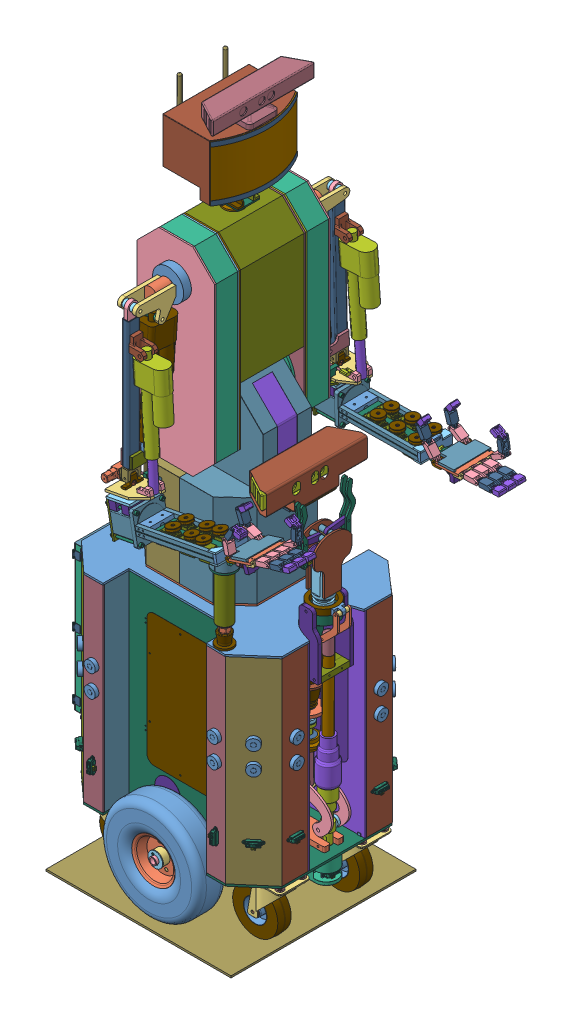
SolidWorks assembly sorbot, configuration По умолчанию. Lengths in mm. (continued)
Mates (geometry in assembly coordinates): (continued)
- Совпадение1280: coincident aligned: plane of SY42STH47-1 through (-54.9903 1468.2936 -152.0542) normal (-1 0 0); plane of head.tilit.p5-1 through (-54.9903 1505.5936 -152.0542) normal (-1 0 0)
- Совпадение1281: coincident anti-aligned: plane of SY42STH47-1 through (-54.9903 1463.2936 -152.0542) normal (0 0 1); plane of head.tilit.p5-1 through (30.0097 1463.2936 -152.0542) normal (0 0 -1)
- Совпадение1283: coincident aligned: plane of head.p1-1 through (-54.9903 1458.2936 -105.9254) normal (-1 0 0); plane of head.tilit.p5-1 through (-54.9903 1505.5936 -152.0542) normal (-1 0 0)
- Заблокировать606: lock: unknown of head.tilt.p1-1; unknown of head.p1-1
- Параллельность222: parallel aligned: plane of body.frame.p2-1 through (92.5097 1112.7235 -222.3642) normal (1 0 0); plane of head.p1-1 through (30.0097 1458.2936 -105.9254) normal (1 0 0)
- Расстояние32: distance = 0.4 mm aligned: plane of head.tilt.p8-1 through (-4.1768 1486.067 -134.1542) normal (0 0 1); plane of head.tilt.p2-1 through (-33.8403 1484.4436 -134.5542) normal (0 0 1)
- Концентричный711: concentric anti-aligned: cylinder of head.tilt.p8-1 through (-4.1768 1486.067 -139.0542) axis (0 0 1) radius 3; cylinder of head.tilt.p9-1 through (-4.1768 1486.067 -112.7074) axis (0 0 -1) radius 3
- Совпадение1286: coincident anti-aligned: plane of head.p1-1 through (30.0097 1458.2936 -164.0542) normal (0 1 0); plane of head.tilit.p5.m-1 through (-54.9903 1458.2936 -121.9254) normal (0 -1 0)
- Совпадение1287: coincident aligned: plane of head.p1-1 through (-54.9903 1458.2936 -105.9254) normal (-1 0 0); plane of head.tilit.p5.m-1 through (-54.9903 1505.5936 -117.9254) normal (-1 0 0)
- Концентричный713: concentric anti-aligned: cylinder of head.tilt.p8-1 through (-4.1768 1486.067 -141.0542) axis (0 0 1) radius 4.85; cylinder of head.tilt.p10-1 through (-4.1768 1486.067 -138.0542) axis (0 0 -1) radius 4.85
- Совпадение1288: coincident anti-aligned: plane of head.tilt.p8-1 through (-4.1768 1486.067 -138.0542) normal (0 0 -1); plane of head.tilt.p10-1 through (-4.1768 1486.067 -138.0542) normal (0 0 1)
- Концентричный714: concentric anti-aligned: cylinder of head.tilt.p8-1 through (-4.1768 1486.067 -132.1542) axis (0 0 -1) radius 4.85; cylinder of head.tilt.p10-2 through (-4.1768 1486.067 -135.1542) axis (0 0 1) radius 4.85
- Совпадение1289: coincident anti-aligned: plane of head.tilt.p8-1 through (-4.1768 1486.067 -135.1542) normal (0 0 1); plane of head.tilt.p10-2 through (-4.1768 1486.067 -135.1542) normal (0 0 -1)
- Концентричный715: concentric anti-aligned: cylinder of head.tilt.p10-2 through (-4.1768 1486.067 -135.1542) axis (0 0 1) radius 4.85; cylinder of head.tilit.p11-1 through (-4.1768 1486.067 -128.1542) axis (0 0 -1) radius 1
- Совпадение1290: coincident anti-aligned: plane of head.tilt.p10-2 through (-4.1768 1486.067 -131.6542) normal (0 0 1); plane of head.tilit.p11-1 through (-6.8677 1566.0217 -131.6542) normal (0 0 -1)
- Концентричный716: concentric aligned: cylinder of head.tilt.p10-1 through (-4.1768 1486.067 -138.0542) axis (0 0 -1) radius 4.85; cylinder of head.tilit.p11-2 through (-4.1768 1486.067 -141.5542) axis (0 0 -1) radius 1
- Совпадение1291: coincident anti-aligned: plane of head.tilt.p10-1 through (-4.1768 1486.067 -141.5542) normal (0 0 -1); plane of head.tilit.p11-2 through (-6.8677 1566.0217 -141.5542) normal (0 0 1)
- Совпадение1292: coincident aligned: plane of head.tilit.p11-1 through (8.1238 1566.5263 -128.1542) normal (0.99746 0.071224 0); plane of head.tilit.p11-2 through (8.1238 1566.5263 -141.5542) normal (0.99746 0.071224 0)
- Заблокировать608: lock: unknown of head.tilt.p8-1; unknown of head.tilt.p10-2
- Заблокировать609: lock: unknown of head.tilt.p8-1; unknown of head.tilt.p10-1
- Заблокировать610: lock: unknown of head.tilt.p10-1; unknown of head.tilit.p11-2
- Заблокировать611: lock: unknown of head.tilt.p10-2; unknown of head.tilit.p11-1
- Концентричный718: concentric anti-aligned: cylinder of head.tilit.p5-1 through (-4.1768 1486.067 -164.0542) axis (0 0 1) radius 3; cylinder of head.tilt.p9-1 through (-4.1768 1486.067 -112.7074) axis (0 0 -1) radius 3
- Концентричный720: concentric aligned: cylinder of head.tilt.p9-1 through (-4.1768 1486.067 -112.7074) axis (0 0 -1) radius 3; cylinder of head.tilt.p12-2 through (-4.1768 1486.067 -145.0542) axis (0 0 -1) radius 3
- Совпадение1294: coincident anti-aligned: plane of head.tilit.p5-1 through (30.0097 1458.2936 -148.0542) normal (0 0 1); plane of head.tilt.p12-2 through (-4.1768 1486.067 -148.0542) normal (0 0 -1)
- Концентричный721: concentric anti-aligned: cylinder of head.tilit.p11-1 through (5.0356 1476.8947 -128.1542) axis (0 0 -1) radius 2; cylinder of m4.nut-5 through (5.0356 1476.8947 -128.1542) axis (0 0 1) radius 2
- Концентричный723: concentric anti-aligned: cylinder of head.tilit.p11-1 through (-4.1485 1473.067 -128.1542) axis (0 0 -1) radius 2; cylinder of m4.nut-6 through (-4.1485 1473.067 -128.1542) axis (0 0 1) radius 2
- Концентричный724: concentric anti-aligned: cylinder of head.tilit.p11-1 through (-13.3492 1476.8546 -128.1542) axis (0 0 -1) radius 2; cylinder of m4.nut-7 through (-13.3492 1476.8546 -128.1542) axis (0 0 1) radius 2
- Концентричный725: concentric anti-aligned: cylinder of head.tilit.p11-1 through (4.9956 1495.2794 -128.1542) axis (0 0 -1) radius 2; cylinder of m4.nut-3 through (4.9956 1495.2794 -128.1542) axis (0 0 1) radius 2
- Концентричный726: concentric anti-aligned: cylinder of head.tilit.p11-1 through (-4.2051 1499.067 -128.1542) axis (0 0 -1) radius 2; cylinder of m4.nut-4 through (-4.2051 1499.067 -128.1542) axis (0 0 1) radius 2
- Концентричный727: concentric anti-aligned: cylinder of head.tilit.p11-1 through (-13.3892 1495.2394 -128.1542) axis (0 0 -1) radius 2; cylinder of m4.nut-8 through (-13.3892 1495.2394 -128.1542) axis (0 0 1) radius 2
- Совпадение1295: coincident anti-aligned: plane of head.tilit.p11-1 through (-6.8677 1566.0217 -128.1542) normal (0 0 1); plane of m4.nut-8 through (-13.3892 1499.2 -128.1542) normal (0 0 -1)
- Совпадение1296: coincident anti-aligned: plane of head.tilit.p11-1 through (-6.8677 1566.0217 -128.1542) normal (0 0 1); plane of m4.nut-4 through (-4.2051 1503.0276 -128.1542) normal (0 0 -1)
- Совпадение1297: coincident anti-aligned: plane of head.tilit.p11-1 through (-6.8677 1566.0217 -128.1542) normal (0 0 1); plane of m4.nut-3 through (4.9956 1499.24 -128.1542) normal (0 0 -1)
- Совпадение1298: coincident anti-aligned: plane of head.tilit.p11-1 through (-6.8677 1566.0217 -128.1542) normal (0 0 1); plane of m4.nut-7 through (-13.3492 1480.8153 -128.1542) normal (0 0 -1)
- Совпадение1299: coincident anti-aligned: plane of head.tilit.p11-1 through (-6.8677 1566.0217 -128.1542) normal (0 0 1); plane of m4.nut-6 through (-4.1485 1477.0277 -128.1542) normal (0 0 -1)
- Совпадение1300: coincident anti-aligned: plane of head.tilit.p11-1 through (-6.8677 1566.0217 -128.1542) normal (0 0 1); plane of m4.nut-5 through (5.0356 1480.8553 -128.1542) normal (0 0 -1)
- Концентричный728: concentric aligned: cylinder of head.tilt.p9-1 through (-4.1768 1486.067 -112.7074) axis (0 0 -1) radius 3; cylinder of m6.washer-7 through (-4.1768 1486.067 -116.2254) axis (0 0 -1) radius 3.25
- Совпадение1301: coincident anti-aligned: plane of head.tilit.p5.m-1 through (-54.9903 1463.2936 -117.9254) normal (0 0 1); plane of m6.washer-7 through (-4.1768 1486.067 -117.9254) normal (0 0 -1)
- Концентричный729: concentric anti-aligned: cylinder of head.tilt.p9-1 through (-4.1768 1486.067 -112.7074) axis (0 0 -1) radius 3; cylinder of m6.washer-8 through (-4.1768 1486.067 -153.7542) axis (0 0 1) radius 3.25
- Совпадение1302: coincident anti-aligned: plane of head.tilit.p5-1 through (30.0097 1463.2936 -152.0542) normal (0 0 -1); plane of m6.washer-8 through (-4.1768 1486.067 -152.0542) normal (0 0 1)
- Заблокировать612: lock: unknown of head.tilit.p5-1; unknown of head.tilt.p9-1
- Концентричный730: concentric aligned: cylinder of head.tilt.p9-1 through (-4.1768 1486.067 -112.7074) axis (0 0 -1) radius 3; cylinder of head.tilt.p12.m-1 through (-4.1768 1486.067 -121.6542) axis (0 0 -1) radius 3
- Совпадение1303: coincident anti-aligned: plane of head.tilit.p11-1 through (-6.8677 1566.0217 -128.1542) normal (0 0 1); plane of head.tilt.p12.m-1 through (-4.1768 1486.067 -128.1542) normal (0 0 -1)
- Совпадение1304: coincident aligned: plane of head.p1-1 through (-54.9903 1458.2936 -105.9254) normal (0 0 1); plane of head.tilit.p5.m-1 through (-54.9903 1463.2936 -105.9254) normal (0 0 1)
- Совпадение1305: coincident aligned: plane of head.p1-1 through (-54.9903 1458.2936 -164.0542) normal (0 0 -1); plane of head.tilit.p5-1 through (30.0097 1463.2936 -164.0542) normal (0 0 -1)
- Концентричный731: concentric anti-aligned: cylinder of head.tilit.p11-1 through (-6.8677 1566.0217 -128.1542) axis (0 0 -1) radius 15; cylinder of head.tilt.p13-1 through (-6.8677 1566.0217 -183.9806) axis (0 0 1) radius 15
- Совпадение1306: coincident anti-aligned: plane of head.tilit.p11-1 through (-6.8677 1566.0217 -131.6542) normal (0 0 -1); plane of head.tilt.p13-1 through (-6.8677 1566.0217 -131.6542) normal (0 0 1)
- Концентричный732: concentric aligned: cylinder of head.p3-1 through (-6.8677 1566.0217 -114.1542) axis (0 0 -1) radius 15.102; cylinder of head.tilit.p11-1 through (-6.8677 1566.0217 -128.1542) axis (0 0 -1) radius 15
- Совпадение1307: coincident anti-aligned: plane of head.tilit.p11-1 through (-6.8677 1566.0217 -128.1542) normal (0 0 1); plane of head.p3-1 through (-21.8677 1551.1571 -128.1542) normal (0 0 -1)
- Концентричный733: concentric anti-aligned: cylinder of head.tilit.p11-2 through (-6.8677 1566.0217 -141.5542) axis (0 0 -1) radius 15; cylinder of head.p3-2 through (-6.8677 1566.0217 -159.0542) axis (0 0 1) radius 15.102
- Совпадение1308: coincident anti-aligned: plane of head.tilit.p11-2 through (-6.8677 1566.0217 -145.0542) normal (0 0 -1); plane of head.p3-2 through (8.1323 1551.1571 -145.0542) normal (0 0 1)
- Совпадение1309: coincident anti-aligned: plane of head.tilit.p11-2 through (-6.8677 1566.0217 -145.0542) normal (0 0 -1); plane of head.p2-1 through (-23.5768 1549.1571 -145.0542) normal (0 0 1)
- Совпадение1311: coincident anti-aligned: plane of head.p3-1 through (-21.8677 1549.1571 -126.1542) normal (0 -1 0); plane of head.p2-1 through (38.3461 1549.1571 -213.999) normal (0 1 0)
- Совпадение1312: coincident: plane of head.tilit.p11-1 through (8.1238 1566.5263 -128.1542) normal (0.99746 0.071224 0); line of head.p2-1 through (9.3641 1549.1571 -128.0542) axis (0 0 -1)
- Заблокировать614: lock: unknown of head.tilit.p11-1; unknown of head.p3-1
- Заблокировать615: lock: unknown of head.tilit.p11-2; unknown of head.p3-2
- Заблокировать616: lock: unknown of head.p2-1; unknown of logitech.sphere.af-1
- Заблокировать617: lock: unknown of head.p2-1; unknown of logitech.sphere.af-2
- Параллельность225: parallel aligned: plane of head.p2-1 through (39.4049 1529.1684 -213.999) normal (0 1 0); plane of head.glass-1 through (-136.7624 1647.1684 -136.5542) normal (0 1 0)
- Расстояние33: distance = 30 mm aligned: plane of head.p2-1 through (39.4049 1527.1684 -213.999) normal (0 -1 0); plane of head.glass-1 through (-136.7624 1497.1684 -136.5542) normal (0 -1 0)
- Концентричный735: concentric aligned: cylinder of head.p2-1 through (23.3461 1547.1571 -198.999) axis (0 1 0) radius 5; circle of logitech.sphere.af-2
- Концентричный736: concentric aligned: cylinder of head.p2-1 through (23.3461 1547.1571 -74.1093) axis (0 1 0) radius 5; circle of logitech.sphere.af-1
- Касательный55: tangent aligned: unknown of logitech.sphere.af-2; cylinder of head.glass-1 through (-136.7624 1647.1684 -136.5542) axis (0 -1 0) radius 211.7321
- Касательный56: tangent aligned: unknown of logitech.sphere.af-1; cylinder of head.glass-1 through (-136.7624 1647.1684 -136.5542) axis (0 -1 0) radius 211.7321
- Расстояние34: distance = 38.4 mm: plane of head.p2-1 through (-26.0264 1529.1684 -59.1093) normal (0 0 1); line of head.glass-1 through (40.4676 1647.1684 -20.7093) axis (0 -1 0)
- Заблокировать618: lock: unknown of head.p2-1; unknown of head.glass-1
- Параллельность226: parallel aligned: plane of head.p1-1 through (30.0097 1458.2936 -105.9254) normal (1 0 0); plane of head.p2-1 through (38.3461 1549.1571 -59.1093) normal (1 0 0)
- Концентричный737: concentric anti-aligned: cylinder of head.glass-1 through (-137.8212 1667.1571 -136.5542) axis (0 -1 0) radius 214.7321; cylinder of head.glass.fixture-1 through (-137.8213 1517.1571 -136.5542) axis (0 1 0) radius 214.7321
- Концентричный738: concentric anti-aligned: cylinder of head.glass-1 through (-137.8212 1667.1571 -136.5542) axis (0 -1 0) radius 214.7321; cylinder of head.glass.fixture-2 through (-137.8212 1655.1571 -136.5542) axis (0 1 0) radius 214.7321
- Совпадение1313: coincident aligned: plane of head.glass-1 through (-137.8212 1667.1571 -136.5542) normal (0 1 0); plane of head.glass.fixture-2 through (-137.8212 1667.1571 -136.5542) normal (0 1 0)
- Совпадение1314: coincident aligned: plane of head.glass-1 through (41.9199 1667.1571 -19.0679) normal (-0.547129 0 0.837048); plane of head.glass.fixture-2 through (41.9199 1655.1571 -19.0679) normal (-0.547129 0 0.837048)
- Совпадение1315: coincident aligned: plane of head.glass-1 through (-137.8213 1517.1571 -136.5542) normal (0 -1 0); plane of head.glass.fixture-1 through (-137.8213 1517.1571 -136.5542) normal (0 -1 0)
- Совпадение1316: coincident aligned: plane of head.glass-1 through (41.9199 1667.1571 -19.0679) normal (-0.547129 0 0.837048); plane of head.glass.fixture-1 through (41.9199 1517.1571 -19.0679) normal (-0.547129 0 0.837048)
- Концентричный739: concentric anti-aligned: cylinder of head.glass-1 through (-137.8212 1667.1571 -136.5542) axis (0 -1 0) radius 211.7321; cylinder of head.p4-1 through (-137.8213 1517.1571 -136.5542) axis (0 1 0) radius 211.73
- Совпадение1317: coincident aligned: plane of head.glass-1 through (-137.8213 1517.1571 -136.5542) normal (0 -1 0); plane of head.p4-1 through (-137.8213 1517.1571 -136.5542) normal (0 -1 0)
- Заблокировать619: lock: unknown of head.p2-1; unknown of head.p4-1
- Совпадение1319: coincident anti-aligned: plane of head.p4-1 through (-84.6104 1578.1571 -252.4244) normal (-1 0 0); plane of ant-3 through (-84.6104 1643.7707 -74.539) normal (1 0 0)
- Совпадение1321: coincident anti-aligned: plane of head.p4-1 through (-84.6104 1578.1571 -252.4244) normal (-1 0 0); plane of ant-2 through (-84.6104 1643.7707 -198.1028) normal (1 0 0)
- Параллельность229: parallel aligned: plane of head.p4-1 through (39.3896 1666.1571 -253.5244) normal (0 0 -1); plane of ant-2 through (-96.1462 1641.4075 -199.6028) normal (0 0 -1)
- Параллельность230: parallel aligned: plane of head.p4-1 through (39.3896 1666.1571 -253.5244) normal (0 0 -1); plane of ant-3 through (-96.1462 1641.4075 -76.039) normal (0 0 -1)
- Заблокировать622: lock: unknown of ant-3; unknown of head.p4-1
- Заблокировать623: lock: unknown of head.p4-1; unknown of ant-2
- Параллельность231: parallel: plane of kinect-black-1 through (-305.9508 1681.1571 -96.5839) normal (0 0 1); plane of head.p4-1 through (-86.6104 1667.1571 -19.5839) normal (0 0 1)
- Совпадение1322: coincident: plane of head.p4-1 through (-137.3095 1668.1571 -136.5542) normal (0 1 0); plane of kinect-black-1 through (-305.9508 1668.1571 -166.5839) normal (0 -1 0)
- Расстояние35: distance = 77 mm aligned: plane of kinect-black-1 through (-305.9508 1681.1571 -96.5839) normal (0 0 1); plane of head.p4-1 through (-86.6104 1667.1571 -19.5839) normal (0 0 1)
- Заблокировать624: lock: unknown of head.p4-1; unknown of kinect-black-1
- Параллельность232: parallel aligned: plane of wall11-1 through (-275.9003 882.565 11.9312) normal (-1 0 0); plane of turret.table-1 through (-172.5648 612.7934 -218.9555) normal (-1 0 0)
- Совпадение1329: coincident aligned: plane of body_pivot-2 through (-90.0648 982.0246 -71.9555) normal (0 0 1); plane of body.cover-1 through (-20.0648 1083.2934 -71.9555) normal (0 0 1)
- Расстояние43: distance = 470 mm: plane of body.cover-1 through (49.9352 1082.7934 -201.9555) normal (0 -1 0); plane of turret.table-1 through (-20.0648 612.7934 -360.2969) normal (0 1 0)
- Coincident1: coincident anti-aligned: plane of wall6-1 through (267.1742 655.3334 -58.2424) normal (1 0 0); plane of Sharp IR GP2D120-1/Sharp IR Body-1 through (267.1742 145.9368 -37.6736) normal (-1 0 0)
- Distance2: distance = 94 mm: line of Sharp IR GP2D120-1/Sharp IR Body-1 through (267.1742 145.9368 -28.4236) axis (0 0 -1); line of wall6-1 through (267.1742 51.9368 11.8264) axis (0 0 -1)
- Distance3: distance = 20 mm: line of wall6-1 through (267.1742 585.1505 11.8264) axis (0 -1 0); line of Sharp IR GP2D120-1/Sharp IR Body-1 through (267.1742 158.9368 -8.1736) axis (0 -1 0)
- Distance6: distance = 20 mm: line of wall7-3 through (267.1973 585.1505 -285.6811) axis (0 -1 0); plane of ? through (274.3242 158.9368 -265.6811) normal (0 0 -1)
- Coincident3: coincident anti-aligned: plane of wall7-3 through (267.1973 693.5591 -285.6811) normal (0.650583 0 -0.759435); plane of Sharp IR GP2D120-3/Sharp IR Body-1 through (214.8514 145.9368 -330.5241) normal (-0.650583 0 0.759435)
- Distance7: distance = 94 mm: line of wall7-3 through (267.1973 51.9368 -285.6811) axis (-0.759435 0 -0.650583); plane of Sharp IR GP2D120-3/Sharp IR Body-1 through (241.9064 145.9368 -316.7619) normal (0 -1 0)
- Lock1: lock: unknown of bottom-2; unknown of wall7-1
- Coincident5: coincident anti-aligned: plane of wall7-1 through (184.8921 693.5591 82.4377) normal (0.650583 0 0.759435); plane of Sharp IR GP2D120-4/Sharp IR Body-1 through (236.9707 145.9368 37.8238) normal (-0.650583 0 -0.759435)
- Distance9: distance = 94 mm: line of wall7-1 through (184.8921 51.9368 82.4377) axis (0.759435 0 -0.650583); plane of Sharp IR GP2D120-4/Sharp IR Body-1 through (219.219 145.9368 62.4459) normal (0 -1 0)
- Coincident8: coincident: plane of wall8-2 through (132.798 -0.3194 -356.1821) normal (0 0 -1); plane of ? through (152.9241 165.4368 -356.1821) normal (0 0 1)
- Distance13: distance = 84 mm: line of wall8-2 through (132.798 51.9368 -356.1821) axis (1 0 0); plane of ? through (165.9241 135.9368 -363.3321) normal (0 -1 0)
- Distance14: distance = 19 mm: line of wall7-3 through (184.9241 585.1505 -356.1619) axis (0 -1 0); plane of ? through (165.9241 135.9368 -363.3321) normal (1 0 0)
- Lock2: lock: unknown of wall8-2; unknown of ?
- Lock3: lock: unknown of wall7-3; unknown of Sharp IR GP2D120-3/Sharp IR Body-1
- Lock4: lock: unknown of wall6-3; unknown of ?
- Lock5: lock: unknown of wall6-1; unknown of Sharp IR GP2D120-1/Sharp IR Body-1
- Lock6: lock: unknown of wall7-1; unknown of Sharp IR GP2D120-4/Sharp IR Body-1
- Lock7: lock: unknown of wall8-1; unknown of Sharp IR GP2D120-5/Sharp IR Body-1
- Lock8: lock: unknown of wall8-5; unknown of ?
- Coincident10: coincident: plane of wall8-4 through (-146.6756 -0.3194 82.4522) normal (0 0 1); plane of Sharp IR GP2D120-8/Sharp IR Body-1 through (-167.0366 165.4368 82.4522) normal (0 0 -1)
- Distance17: distance = 84 mm: line of wall8-4 through (-146.6756 51.9368 82.4522) axis (-1 0 0); plane of Sharp IR GP2D120-8/Sharp IR Body-1 through (-180.0366 135.9368 89.6022) normal (0 -1 0)
- Distance18: distance = 19 mm: line of wall7-v1-1 through (-199.0366 51.9368 82.0998) axis (0 1 0); plane of Sharp IR GP2D120-8/Sharp IR Body-1 through (-180.0366 135.9368 89.6022) normal (-1 0 0)
- Lock9: lock: unknown of wall8-4; unknown of Sharp IR GP2D120-8/Sharp IR Body-1
- Coincident11: coincident: plane of wall7-v1-2 through (-275.6816 -52.2153 -285.955) normal (-0.67421 0 -0.73854); plane of Sharp IR GP2D120-9/Sharp IR Body-1 through (-246.8786 145.9368 -312.2492) normal (0.67421 0 0.73854)
- Distance19: distance = 94 mm: plane of Sharp IR GP2D120-9/Sharp IR Body-1 through (-229.9122 145.9368 -337.419) normal (0 -1 0); line of wall7-v1-2 through (-275.6816 51.9368 -285.955) axis (0.73854 0 -0.67421)
- Distance20: distance = 39 mm: line of wall7-v1-2 through (-275.6816 51.9368 -285.955) axis (0 1 0); plane of Sharp IR GP2D120-9/Sharp IR Body-1 through (-251.6992 158.9368 -317.5298) normal (-0.73854 0 0.67421)
- Lock10: lock: unknown of wall7-v1-2; unknown of Sharp IR GP2D120-9/Sharp IR Body-1
- Coincident12: coincident anti-aligned: plane of wall7-v1-1 through (-199.0366 -52.2153 82.0998) normal (-0.67421 0 0.73854); plane of Sharp IR GP2D120-10/Sharp IR Body-1 through (-225.3104 145.9368 58.1146) normal (0.67421 0 -0.73854)
- Distance21: distance = 94 mm: plane of Sharp IR GP2D120-10/Sharp IR Body-1 through (-251.9179 145.9368 43.5059) normal (0 -1 0); line of bottom-2 through (-275.9596 51.9368 11.9714) axis (0.73854 0 0.67421)
- Distance22: distance = 39 mm: line of wall7-v1-1 through (-275.9003 51.9368 11.9312) axis (0 1 0); plane of Sharp IR GP2D120-10/Sharp IR Body-1 through (-251.9179 158.9368 43.5059) normal (-0.73854 0 -0.67421)
- Lock11: lock: unknown of wall7-v1-1; unknown of Sharp IR GP2D120-10/Sharp IR Body-1
- Coincident13: coincident anti-aligned: plane of wall10-v1-1 through (132.8227 864.7556 -286.1821) normal (0 0 -1); plane of wall10.opening.cap-1 through (52.686 120.491 -286.1821) normal (0 0 1)
- Concentric1: concentric aligned: circle of wall10-v1-1; circle of wall10.opening.cap-1
- Coincident14: coincident anti-aligned: plane of wall10-1 through (-146.6756 864.7556 12.4522) normal (0 0 1); plane of wall10.opening.cap-2 through (-41.2841 118.8489 12.4522) normal (0 0 -1)
- Concentric2: concentric aligned: circle of wall10-1; circle of wall10.opening.cap-2
- Coincident15: coincident anti-aligned: plane of wall10-1 through (-146.6756 864.7556 12.4522) normal (0 0 1); plane of wall10-cap-1 through (-77.6414 499.1505 12.4522) normal (0 0 -1)
- Coincident16: coincident anti-aligned: plane of wall10-v1-1 through (132.8227 864.7556 -286.1821) normal (0 0 -1); plane of wall10-cap-2 through (-77.5708 499.1505 -286.1821) normal (0 0 1)
- Coincident17: coincident anti-aligned: plane of wall6-1 through (267.1742 655.3334 -58.2424) normal (1 0 0); plane of us_sensor-1 through (267.1742 386.9368 -23.208) normal (-1 0 0)
- Coincident18: coincident anti-aligned: plane of bottom-2 through (-49.3372 51.9368 -286.1821) normal (0 1 0); plane of wall6-3 through (263.1741 51.9368 -286.3112) normal (0 -1 0)
- Coincident19: coincident aligned: line of wall2-2 through (267.1741 585.1505 -216.2424) axis (0 -1 0); line of wall6-3 through (267.1741 585.1505 -216.2424) axis (0 -1 0)
- Coincident20: coincident aligned: plane of bottom-2 through (267.1742 51.9368 -285.7013) normal (1 0 0); plane of wall6-3 through (267.1741 655.3334 -286.3112) normal (1 0 0)
- Coincident21: coincident anti-aligned: plane of wall6-1 through (267.1742 655.3334 -58.2424) normal (1 0 0); plane of us_sensor-2 through (267.1742 326.9368 -23.208) normal (-1 0 0)
- Concentric3: concentric anti-aligned: cylinder of wall6-1 through (263.1742 386.9368 -23.208) axis (1 0 0) radius 6; cylinder of us_sensor-1 through (277.1742 386.9368 -23.208) axis (-1 0 0) radius 15
- Concentric4: concentric anti-aligned: cylinder of wall6-1 through (263.1742 326.9368 -23.208) axis (1 0 0) radius 6; cylinder of us_sensor-2 through (277.1742 326.9368 -23.208) axis (-1 0 0) radius 15
- Coincident22: coincident anti-aligned: plane of wall6-3 through (267.1742 655.3334 -286.3112) normal (1 0 0); plane of us_sensor-3 through (267.1742 326.9368 -251.2768) normal (-1 0 0)
- Coincident23: coincident anti-aligned: plane of wall6-3 through (267.1742 655.3334 -286.3112) normal (1 0 0); plane of us_sensor-4 through (267.1742 386.9368 -251.2768) normal (-1 0 0)
- Concentric5: concentric anti-aligned: cylinder of wall6-3 through (263.1742 386.9368 -251.2768) axis (1 0 0) radius 6; cylinder of us_sensor-4 through (277.1742 386.9368 -251.2768) axis (-1 0 0) radius 15
- Concentric6: concentric anti-aligned: cylinder of wall6-3 through (263.1742 326.9368 -251.2768) axis (1 0 0) radius 6; cylinder of us_sensor-3 through (277.1742 326.9368 -251.2768) axis (-1 0 0) radius 15
- Coincident24: coincident anti-aligned: plane of bottom-2 through (-49.3372 51.9368 -286.1821) normal (0 1 0); plane of wall8-5 through (-199.1911 51.9368 -356.1821) normal (0 -1 0)
- Coincident26: coincident aligned: plane of bottom-2 through (-146.7539 51.9368 -356.1821) normal (0 0 -1); plane of wall8-5 through (-199.1911 51.9368 -356.1821) normal (0 0 -1)
- Coincident27: coincident aligned: plane of bottom-2 through (-146.7539 51.9368 -286.1821) normal (1 0 0); plane of wall9-3 through (-146.7539 655.1671 -356.1821) normal (1 0 0)
- Lock12: lock: unknown of bottom-2; unknown of wall9-3
- Coincident31: coincident anti-aligned: plane of bottom-2 through (-49.3372 51.9368 -286.1821) normal (0 1 0); plane of wall8-1 through (184.8921 51.9368 82.4377) normal (0 -1 0)
- Coincident32: coincident anti-aligned: line of wall7-1 through (184.8921 585.1505 82.4377) axis (0 -1 0); line of wall8-1 through (184.8921 51.9368 82.4377) axis (0 1 0)
- Coincident34: coincident anti-aligned: plane of wall7-3 through (267.1973 693.5591 -285.6811) normal (0.650583 0 -0.759435); plane of us_sensor-5 through (226.0607 386.9368 -320.9215) normal (-0.650583 0 0.759435)
- Coincident35: coincident anti-aligned: plane of wall7-3 through (267.1973 693.5591 -285.6811) normal (0.650583 0 -0.759435); plane of us_sensor-6 through (226.0607 326.9368 -320.9215) normal (-0.650583 0 0.759435)
- Concentric7: concentric anti-aligned: cylinder of wall7-3 through (223.4584 386.9368 -317.8837) axis (0.650583 0 -0.759435) radius 6; cylinder of us_sensor-5 through (232.5665 386.9368 -328.5158) axis (-0.650583 0 0.759435) radius 15
- Concentric8: concentric anti-aligned: cylinder of wall7-3 through (223.4584 326.9368 -317.8837) axis (0.650583 0 -0.759435) radius 6; cylinder of us_sensor-6 through (232.5665 326.9368 -328.5158) axis (-0.650583 0 0.759435) radius 15
- Coincident36: coincident anti-aligned: plane of wall8-2 through (132.798 51.9368 -356.1821) normal (0 0 -1); plane of us_sensor-8 through (158.8495 386.9368 -356.1821) normal (0 0 1)
- Coincident37: coincident: plane of wall8-2 through (132.798 51.9368 -356.1821) normal (0 0 -1); plane of us_sensor-7 through (158.8495 326.9368 -356.1821) normal (0 0 1)
- Concentric9: concentric anti-aligned: cylinder of wall8-2 through (158.8495 386.9368 -352.1821) axis (0 0 -1) radius 6; cylinder of us_sensor-8 through (158.8495 386.9368 -366.1821) axis (0 0 1) radius 15
- Concentric10: concentric anti-aligned: cylinder of wall8-2 through (158.8495 326.9368 -352.1821) axis (0 0 -1) radius 6; cylinder of us_sensor-7 through (158.8495 326.9368 -366.1821) axis (0 0 1) radius 15
- Coincident38: coincident: plane of wall8-5 through (-199.1911 51.9368 -356.1821) normal (0 0 -1); plane of us_sensor-10 through (-173.1397 386.9368 -356.1821) normal (0 0 1)
- Coincident39: coincident: plane of wall8-5 through (-199.1911 51.9368 -356.1821) normal (0 0 -1); plane of us_sensor-9 through (-173.1397 326.9368 -356.1821) normal (0 0 1)
- Concentric11: concentric anti-aligned: cylinder of wall8-5 through (-173.1397 386.9368 -352.1821) axis (0 0 -1) radius 6; cylinder of us_sensor-10 through (-173.1397 386.9368 -366.1821) axis (0 0 1) radius 15
- Concentric12: concentric anti-aligned: cylinder of wall8-5 through (-173.1397 326.9368 -352.1821) axis (0 0 -1) radius 6; cylinder of us_sensor-9 through (-173.1397 326.9368 -366.1821) axis (0 0 1) radius 15
- Coincident40: coincident: plane of wall7-v1-2 through (-275.6816 -52.2153 -285.955) normal (-0.67421 0 -0.73854); plane of us_sensor-12 through (-237.2497 386.9368 -321.0393) normal (0.67421 0 0.73854)
- Coincident41: coincident: plane of wall7-v1-2 through (-275.6816 -52.2153 -285.955) normal (-0.67421 0 -0.73854); plane of us_sensor-11 through (-237.2497 326.9368 -321.0393) normal (0.67421 0 0.73854)
- Concentric13: concentric anti-aligned: cylinder of wall7-v1-2 through (-234.5529 386.9368 -318.0852) axis (-0.67421 0 -0.73854) radius 6; cylinder of us_sensor-12 through (-243.9918 386.9368 -328.4247) axis (0.67421 0 0.73854) radius 15
- Concentric14: concentric anti-aligned: cylinder of wall7-v1-2 through (-234.5529 326.9368 -318.0852) axis (-0.67421 0 -0.73854) radius 6; cylinder of us_sensor-11 through (-243.9918 326.9368 -328.4247) axis (0.67421 0 0.73854) radius 15
- Coincident42: coincident: plane of wall7-v1-1 through (-199.0366 -52.2153 82.0998) normal (-0.67421 0 0.73854); plane of us_sensor-14 through (-237.4685 386.9368 47.0155) normal (0.67421 0 -0.73854)
- Coincident43: coincident: plane of wall7-v1-1 through (-199.0366 -52.2153 82.0998) normal (-0.67421 0 0.73854); plane of us_sensor-13 through (-237.4685 326.9368 47.0155) normal (0.67421 0 -0.73854)
- Concentric15: concentric anti-aligned: cylinder of wall7-v1-1 through (-234.7716 386.9368 44.0613) axis (-0.67421 0 0.73854) radius 6; cylinder of us_sensor-14 through (-244.2106 386.9368 54.4009) axis (0.67421 0 -0.73854) radius 15
- Concentric16: concentric anti-aligned: cylinder of wall7-v1-1 through (-234.7716 326.9368 44.0613) axis (-0.67421 0 0.73854) radius 6; cylinder of us_sensor-13 through (-244.2106 326.9368 54.4009) axis (0.67421 0 -0.73854) radius 15
- Coincident44: coincident: plane of wall8-4 through (-146.6756 51.9505 82.4522) normal (0 0 1); plane of us_sensor-16 through (-172.7271 386.9505 82.4522) normal (0 0 -1)
- Coincident45: coincident: plane of wall8-4 through (-146.6756 51.9505 82.4522) normal (0 0 1); plane of us_sensor-15 through (-172.7271 326.9505 82.4522) normal (0 0 -1)
- Concentric17: concentric anti-aligned: cylinder of wall8-4 through (-172.7271 386.9505 78.4522) axis (0 0 1) radius 6; cylinder of us_sensor-16 through (-172.7271 386.9505 92.4522) axis (0 0 -1) radius 15
- Concentric18: concentric anti-aligned: cylinder of wall8-4 through (-172.7271 326.9505 78.4522) axis (0 0 1) radius 6; cylinder of us_sensor-15 through (-172.7271 326.9505 92.4522) axis (0 0 -1) radius 15
- Coincident46: coincident: plane of wall8-1 through (184.8921 51.9368 82.4377) normal (-0.006017 0 0.999982); plane of us_sensor-18 through (158.8412 386.9368 82.281) normal (0.006017 0 -0.999982)
- Coincident47: coincident: plane of wall8-1 through (184.8921 51.9368 82.4377) normal (-0.006017 0 0.999982); plane of us_sensor-17 through (158.8412 326.9368 82.281) normal (0.006017 0 -0.999982)
- Concentric19: concentric anti-aligned: cylinder of wall8-1 through (158.8652 386.9368 78.281) axis (-0.006017 0 0.999982) radius 6; cylinder of us_sensor-18 through (158.781 386.9368 92.2808) axis (0.006017 0 -0.999982) radius 15
- Concentric20: concentric anti-aligned: cylinder of wall8-1 through (158.8652 326.9368 78.281) axis (-0.006017 0 0.999982) radius 6; cylinder of us_sensor-17 through (158.781 326.9368 92.2808) axis (0.006017 0 -0.999982) radius 15
- Coincident48: coincident: plane of wall7-1 through (184.8921 693.5591 82.4377) normal (0.650583 0 0.759435); plane of us_sensor-20 through (226.0288 386.9368 47.1973) normal (-0.650583 0 -0.759435)
- Coincident49: coincident: plane of wall7-1 through (184.8921 693.5591 82.4377) normal (0.650583 0 0.759435); plane of us_sensor-19 through (226.0288 326.9368 47.1973) normal (-0.650583 0 -0.759435)
- Concentric21: concentric anti-aligned: cylinder of wall7-1 through (223.4265 386.9368 44.1596) axis (0.650583 0 0.759435) radius 6; cylinder of us_sensor-20 through (232.5346 386.9368 54.7917) axis (-0.650583 0 -0.759435) radius 15
- Concentric22: concentric anti-aligned: cylinder of wall7-1 through (223.4265 326.9368 44.1596) axis (0.650583 0 0.759435) radius 6; cylinder of us_sensor-19 through (232.5346 326.9368 54.7917) axis (-0.650583 0 -0.759435) radius 15
- Lock13: lock: unknown of wall6-3; unknown of us_sensor-4
- Lock14: lock: unknown of wall6-3; unknown of us_sensor-3
- Lock15: lock: unknown of wall7-3; unknown of us_sensor-5
- Lock16: lock: unknown of wall7-3; unknown of us_sensor-6
- Lock17: lock: unknown of wall8-2; unknown of us_sensor-8
- Lock18: lock: unknown of wall8-2; unknown of us_sensor-7
- Lock19: lock: unknown of wall8-5; unknown of us_sensor-10
- Lock20: lock: unknown of wall8-5; unknown of us_sensor-9
- Lock21: lock: unknown of wall7-v1-2; unknown of us_sensor-12
- Lock22: lock: unknown of wall7-v1-2; unknown of us_sensor-11
- Lock23: lock: unknown of wall7-v1-1; unknown of us_sensor-14
- Lock24: lock: unknown of wall7-v1-1; unknown of us_sensor-13
- Lock25: lock: unknown of wall8-4; unknown of us_sensor-16
- Lock26: lock: unknown of wall8-4; unknown of us_sensor-15
- Lock27: lock: unknown of wall8-1; unknown of us_sensor-18
- Lock28: lock: unknown of wall8-1; unknown of us_sensor-17
- Lock29: lock: unknown of wall7-1; unknown of us_sensor-20
- Lock30: lock: unknown of wall7-1; unknown of us_sensor-19
- Lock31: lock: unknown of wall6-1; unknown of us_sensor-1
- Lock32: lock: unknown of wall6-1; unknown of us_sensor-2
- Coincident50: coincident: plane of wall11-1 through (-271.9003 882.565 10.1667) normal (1 0 0); plane of computer.box.hinge-1 through (-271.9003 559.9368 -55.5688) normal (-1 0 0)
- Coincident51: coincident: plane of wall11-1 through (-271.9003 882.565 10.1667) normal (1 0 0); plane of computer.box.hinge-2 through (-271.9003 559.9368 -217.9564) normal (-1 0 0)
- Coincident52: coincident: point of wall11-1; unknown of computer.box.hinge-2
- Coincident53: coincident: unknown of wall11-1; unknown of computer.box.hinge-1
- Lock33: lock: unknown of wall11-1; unknown of computer.box.hinge-1
- Lock34: lock: unknown of wall11-1; unknown of computer.box.hinge-2
- Lock36: lock: unknown of computer.box.hinge-2; unknown of computer.box.console-1/computer.box.fixture.console-1
- Coincident58: coincident anti-aligned: plane of wall11-1 through (-271.9003 556.9368 -38.0688) normal (0 1 0); plane of computer.box.console-2/cap-hinge-p1-1 through (-280.8434 556.9368 -36.0276) normal (0 -1 0)
- Lock37: lock: unknown of computer.box.hinge-1; unknown of computer.box.console-2/computer.box.fixture.console-1
- Concentric23: concentric anti-aligned: cylinder of computer.box.console-2/cap-hinge-p1-1 through (-280.8434 559.9368 -36.0276) axis (0 0 -1) radius 2; cylinder of computer.box.base-1/cap-hinge-2 through (-280.8434 559.9368 -75.2651) axis (0 0 1) radius 2
- Coincident60: coincident anti-aligned: plane of computer.box.console-2/cap-hinge-p1-1 through (-275.9003 539.9368 -65.2651) normal (0 0 -1); plane of computer.box.base-1/cap-hinge-2 through (-260.8434 565.7704 -65.2651) normal (0 0 1)
- Coincident67: coincident anti-aligned: plane of computer.box.base-1/computer.box.cap.hinge.p2-1 through (-311.8434 354.9938 -4.6907) normal (0 -1 0); plane of computer.box.cap-1/computer.box.cap.hinge.p1-2 through (-317.3839 354.9938 1.7687) normal (0 1 0)
- Concentric27: concentric anti-aligned: cylinder of computer.box.base-1/computer.box.cap.hinge.p2-1 through (-315.7839 349.9938 -6.2907) axis (0 1 0) radius 1; cylinder of computer.box.cap-1/computer.box.cap.hinge.p1-2 through (-315.7839 369.9938 -6.2907) axis (0 -1 0) radius 1
- Parallel2: parallel aligned: plane of wall11-1 through (-275.9003 882.565 11.9312) normal (-1 0 0); unknown of computer.box.cap-1/computer.box.cap.base-1
- Lock39: lock: unknown of computer.box.base-1/computer.box.corner.p1-2; unknown of computer.box.cap-1/computer.box.cap.base-1
- Parallel1: parallel anti-aligned: plane of wall11-1 through (-275.9003 882.565 11.9312) normal (-1 0 0); plane of computer.box.base-1/computer.box.bottom-1 through (-281.8434 357.9938 -137.7651) normal (1 0 0)
- Coincident68: coincident anti-aligned: plane of bottom-2 through (-49.3372 51.9368 -286.1821) normal (0 1 0); plane of accumulator.5Ah-2 through (-152.9596 51.9368 -134.0478) normal (0 -1 0)
- Parallel3: parallel aligned: plane of bottom-2 through (-275.9596 51.9368 -285.7013) normal (-1 0 0); plane of accumulator.5Ah-2 through (-235.9596 53.9368 -68.0478) normal (-1 0 0)
- Distance23: distance = 40 mm aligned: plane of bottom-2 through (-275.9596 51.9368 -285.7013) normal (-1 0 0); plane of accumulator.5Ah-2 through (-235.9596 53.9368 -68.0478) normal (-1 0 0)
- Distance24: distance = 148.5 mm aligned: plane of bottom-2 through (-146.7539 51.9368 82.4522) normal (0 0 1); plane of accumulator.5Ah-2 through (-152.9596 139.9368 -66.0478) normal (0 0 1)
- Coincident69: coincident anti-aligned: plane of bottom-2 through (-49.3372 51.9368 -286.1821) normal (0 1 0); plane of accumulator.5Ah-1 through (-152.9596 51.9368 -205.6821) normal (0 -1 0)
- Distance25: distance = 40 mm aligned: plane of accumulator.5Ah-1 through (-235.9596 53.9368 -139.6821) normal (-1 0 0); plane of bottom-2 through (-275.9596 51.9368 -285.7013) normal (-1 0 0)
- Distance26: distance = 148.5 mm aligned: plane of accumulator.5Ah-1 through (-152.9596 139.9368 -207.6821) normal (0 0 -1); plane of bottom-2 through (-146.7539 51.9368 -356.1821) normal (0 0 -1)
- Parallel4: parallel aligned: plane of bottom-2 through (-275.9596 51.9368 -285.7013) normal (-1 0 0); plane of accumulator.loft-1 through (-270.9596 147.9368 -244.8821) normal (-1 0 0)
- Distance27: distance = 91 mm anti-aligned: plane of accumulator.loft-1 through (-267.9596 142.9368 -244.8821) normal (0 -1 0); plane of bottom-2 through (-49.3372 51.9368 -286.1821) normal (0 1 0)
- Distance28: distance = 108.3 mm aligned: plane of bottom-2 through (-146.7539 51.9368 -356.1821) normal (0 0 -1); plane of accumulator.loft-1 through (-108.9596 147.9368 -247.8821) normal (0 0 -1)
- Distance29: distance = 5 mm aligned: plane of bottom-2 through (-275.9596 51.9368 -285.7013) normal (-1 0 0); plane of accumulator.loft-1 through (-270.9596 147.9368 -244.8821) normal (-1 0 0)
- Coincident70: coincident anti-aligned: plane of accumulator.loft-1 through (-267.9596 142.9368 -244.8821) normal (0 -1 0); plane of accumulator.loft.pillar-1 through (-117.9596 142.9368 -39.8821) normal (0 1 0)
- Coincident71: coincident anti-aligned: plane of accumulator.loft-1 through (-267.9596 142.9368 -244.8821) normal (0 -1 0); plane of accumulator.loft.pillar-2 through (-225.9596 142.9368 -39.8821) normal (0 1 0)
- Coincident72: coincident anti-aligned: plane of accumulator.loft-1 through (-267.9596 142.9368 -244.8821) normal (0 -1 0); plane of accumulator.loft.pillar-3 through (-117.9596 142.9368 -235.8821) normal (0 1 0)
- Coincident73: coincident anti-aligned: plane of accumulator.loft-1 through (-267.9596 142.9368 -244.8821) normal (0 -1 0); plane of accumulator.loft.pillar-4 through (-225.9596 142.9368 -235.8821) normal (0 1 0)
- Concentric28: concentric aligned: cylinder of accumulator.loft-1 through (-117.9596 147.9368 -39.8821) axis (0 -1 0) radius 2.5; cylinder of accumulator.loft.pillar-1 through (-117.9596 142.9368 -39.8821) axis (0 -1 0) radius 3
- Concentric29: concentric aligned: cylinder of accumulator.loft-1 through (-225.9596 147.9368 -39.8821) axis (0 -1 0) radius 2.5; cylinder of accumulator.loft.pillar-2 through (-225.9596 142.9368 -39.8821) axis (0 -1 0) radius 3
- Concentric30: concentric aligned: cylinder of accumulator.loft-1 through (-117.9596 147.9368 -235.8821) axis (0 -1 0) radius 2.5; cylinder of accumulator.loft.pillar-3 through (-117.9596 142.9368 -235.8821) axis (0 -1 0) radius 3
- Concentric31: concentric aligned: cylinder of accumulator.loft-1 through (-225.9596 147.9368 -235.8821) axis (0 -1 0) radius 2.5; cylinder of accumulator.loft.pillar-4 through (-225.9596 142.9368 -235.8821) axis (0 -1 0) radius 3
- Coincident74: coincident anti-aligned: plane of accumulator.loft-1 through (-267.9596 147.9368 -244.8821) normal (0 1 0); plane of accumulator.loft.rubber-1 through (-188.4596 147.9368 -137.8821) normal (0 -1 0)
- Parallel5: parallel aligned: plane of accumulator.loft-1 through (-270.9596 147.9368 -244.8821) normal (-1 0 0); plane of accumulator.loft.rubber-1 through (-269.9596 154.9368 -246.8821) normal (-1 0 0)
- Distance31: distance = 1 mm aligned: plane of accumulator.loft.rubber-1 through (-106.9596 154.9368 -28.8821) normal (0 0 1); plane of accumulator.loft-1 through (-108.9596 147.9368 -27.8821) normal (0 0 1)
- Distance32: distance = 1 mm aligned: plane of accumulator.loft-1 through (-270.9596 147.9368 -244.8821) normal (-1 0 0); plane of accumulator.loft.rubber-1 through (-269.9596 154.9368 -246.8821) normal (-1 0 0)
- Coincident75: coincident anti-aligned: plane of accumulator1-1 through (-270.9596 154.9368 -27.8821) normal (0 -1 0); plane of accumulator.loft.rubber-1 through (-188.4596 154.9368 -137.8821) normal (0 1 0)
- Coincident78: coincident aligned: plane of accumulator1-1 through (-270.9596 320.9368 -247.8821) normal (-1 0 0); plane of accumulator.loft-1 through (-270.9596 147.9368 -244.8821) normal (-1 0 0)
- Coincident79: coincident aligned: plane of accumulator1-1 through (-105.9596 320.9368 -27.8821) normal (0 0 1); plane of accumulator.loft-1 through (-108.9596 147.9368 -27.8821) normal (0 0 1)
- Coincident80: coincident anti-aligned: plane of wall11-1 through (-275.9003 882.565 11.9312) normal (-1 0 0); plane of us_sensor-21 through (-275.9003 565.1505 -170.4564) normal (1 0 0)
- Coincident81: coincident anti-aligned: plane of wall11-1 through (-275.9003 882.565 11.9312) normal (-1 0 0); plane of us_sensor-22 through (-275.9003 565.1505 -103.0688) normal (1 0 0)
- Coincident82: coincident anti-aligned: plane of wall11-1 through (-275.9003 882.565 11.9312) normal (-1 0 0); plane of us_sensor-23 through (-275.9003 146.9368 -170.4564) normal (1 0 0)
- Coincident83: coincident anti-aligned: plane of wall11-1 through (-275.9003 882.565 11.9312) normal (-1 0 0); plane of us_sensor-24 through (-275.9003 146.9368 -103.0688) normal (1 0 0)
- Concentric32: concentric anti-aligned: cylinder of wall11-1 through (-271.9003 570.1505 -170.4564) axis (-1 0 0) radius 6; cylinder of us_sensor-21 through (-285.9003 570.1505 -170.4564) axis (1 0 0) radius 15
- Concentric33: concentric anti-aligned: cylinder of wall11-1 through (-271.9003 570.1505 -103.0688) axis (-1 0 0) radius 6; cylinder of us_sensor-22 through (-285.9003 570.1505 -103.0688) axis (1 0 0) radius 15
- Concentric34: concentric anti-aligned: cylinder of wall11-1 through (-271.9003 146.9368 -170.4564) axis (-1 0 0) radius 6; cylinder of us_sensor-23 through (-285.9003 146.9368 -170.4564) axis (1 0 0) radius 15
- Concentric35: concentric anti-aligned: cylinder of wall11-1 through (-271.9003 146.9368 -103.0688) axis (-1 0 0) radius 6; cylinder of us_sensor-24 through (-285.9003 146.9368 -103.0688) axis (1 0 0) radius 15
- Coincident84: coincident anti-aligned: plane of wall11-1 through (-275.9003 882.565 11.9312) normal (-1 0 0); plane of ? through (-275.9003 145.9368 101.8971) normal (1 0 0)
- Coincident85: coincident anti-aligned: plane of wall11-1 through (-275.9003 882.565 11.9312) normal (-1 0 0); plane of ? through (-275.9003 145.9368 145.8787) normal (1 0 0)
- Parallel6: parallel anti-aligned: plane of bottom-2 through (-49.3372 51.9368 -286.1821) normal (0 1 0); plane of ? through (-283.0503 145.9368 72.3971) normal (0 -1 0)
- Parallel7: parallel anti-aligned: plane of bottom-2 through (-49.3372 51.9368 -286.1821) normal (0 1 0); plane of ? through (-283.0503 145.9368 116.3787) normal (0 -1 0)
- Distance33: distance = 94 mm: line of bottom-2 through (-275.9596 51.9368 -285.7013) axis (0 0 1); plane of Sharp IR GP2D120-11/Sharp IR Body-1 through (-283.0503 145.9368 -245.4564) normal (0 -1 0)
- Distance34: distance = 94 mm: plane of Sharp IR GP2D120-12/Sharp IR Body-1 through (-283.0503 145.9368 -57.5688) normal (0 -1 0); line of bottom-2 through (-275.9596 51.9368 -285.7013) axis (0 0 1)
- Distance35: distance = 40 mm: line of wall11-1 through (-275.9003 585.1505 -285.4564) axis (0 -1 0); plane of Sharp IR GP2D120-11/Sharp IR Body-1 through (-283.0503 158.9368 -245.4564) normal (0 0 -1)
- Distance36: distance = 40 mm: line of wall11-1 through (-275.9003 585.1505 11.9312) axis (0 -1 0); plane of Sharp IR GP2D120-12/Sharp IR Body-1 through (-283.0503 158.9368 -28.0688) normal (0 0 1)
- Lock40: lock: unknown of wall11-1; unknown of us_sensor-21
- Lock41: lock: unknown of wall11-1; unknown of us_sensor-22
- Lock42: lock: unknown of wall11-1; unknown of us_sensor-23
- Lock43: lock: unknown of wall11-1; unknown of us_sensor-24
- Lock44: lock: unknown of wall11-1; unknown of Sharp IR GP2D120-11/Sharp IR Body-1
- Lock45: lock: unknown of wall11-1; unknown of Sharp IR GP2D120-12/Sharp IR Body-1
- Coincident86: coincident: unknown of accumulator.charger.sm1236-1; unknown of pillar.10mm-1
- Coincident87: coincident: unknown of accumulator.charger.sm1236-1; unknown of pillar.10mm-2
- Coincident88: coincident: unknown of accumulator.charger.sm1236-1; unknown of pillar.10mm-3
- Coincident89: coincident: unknown of accumulator.charger.sm1236-1; unknown of pillar.10mm-4
- Concentric36: concentric anti-aligned: cylinder of accumulator.charger.sm1236-1 through (-347.0666 292.9966 -370.5276) axis (0 1 0) radius 2; cylinder of pillar.10mm-2 through (-347.0666 292.9966 -370.5276) axis (0 -1 0) radius 1.5
- Concentric37: concentric anti-aligned: cylinder of accumulator.charger.sm1236-1 through (-347.0666 292.9966 -322.0562) axis (0 1 0) radius 2; cylinder of pillar.10mm-3 through (-347.0666 292.9966 -322.0562) axis (0 -1 0) radius 1.5
- Concentric38: concentric anti-aligned: cylinder of accumulator.charger.sm1236-1 through (-538.5098 292.9966 -312.004) axis (0 1 0) radius 2; cylinder of pillar.10mm-1 through (-538.5098 292.9966 -312.004) axis (0 -1 0) radius 1.5
- Concentric39: concentric anti-aligned: cylinder of accumulator.charger.sm1236-1 through (-538.5098 292.9966 -380.5797) axis (0 1 0) radius 2; cylinder of pillar.10mm-4 through (-538.5098 292.9966 -380.5797) axis (0 -1 0) radius 1.5
- Lock46: lock: unknown of accumulator.charger.sm1236-1; unknown of pillar.10mm-4
- Lock47: lock: unknown of accumulator.charger.sm1236-1; unknown of pillar.10mm-1
- Lock48: lock: unknown of accumulator.charger.sm1236-1; unknown of pillar.10mm-3
- Lock49: lock: unknown of accumulator.charger.sm1236-1; unknown of pillar.10mm-2
- Parallel8: parallel anti-aligned: plane of bottom-2 through (-49.3372 51.9368 -286.1821) normal (0 1 0); plane of accumulator.charger.sm1236-1 through (216.0916 329.8029 -262.3065) normal (0 -1 0)
- Coincident91: coincident anti-aligned: plane of wall-fixture-v1-2 through (-152.6756 584.9368 28.4522) normal (-1 0 0); plane of electic.base.plate-1 through (-152.6756 514.1505 -136.5478) normal (1 0 0)
- Parallel9: parallel aligned: plane of wall9-3 through (-142.2412 585.1505 -459.5586) normal (0 1 0); plane of electic.base.plate-1 through (-157.6756 565.1505 34.4522) normal (0 1 0)
- Distance37: distance = 44 mm anti-aligned: plane of wall8-4 through (-146.6756 51.9505 78.4522) normal (0 0 -1); plane of electic.base.plate-1 through (-157.6756 463.1505 34.4522) normal (0 0 1)
- Distance38: distance = 20 mm anti-aligned: plane of cap-1 through (216.6678 585.1505 -83.5666) normal (0 -1 0); plane of electic.base.plate-1 through (-157.6756 565.1505 34.4522) normal (0 1 0)
- Coincident96: coincident anti-aligned: plane of wall-fixture-v2-1-1 through (-269.9003 624.2006 -10.7109) normal (1 0 0); plane of computer.box.screw.fixture-2 through (-269.9003 548.1505 0.207) normal (-1 0 0)
- Coincident97: coincident anti-aligned: plane of wall-fixture-v2-1-2 through (-269.9003 624.1077 -280.8026) normal (1 0 0); plane of computer.box.screw.fixture-1 through (-269.9003 548.1505 -274.4564) normal (-1 0 0)
- Coincident98: coincident anti-aligned: plane of wall-fixture-v2-1-2 through (-269.9003 624.1077 -280.8026) normal (1 0 0); plane of computer.box.screw.fixture-3 through (-269.9003 171.4368 0.207) normal (-1 0 0)
- Coincident99: coincident anti-aligned: plane of wall-fixture-v2-1-1 through (-267.4772 624.2006 -10.7109) normal (1 0 0); plane of computer.box.screw.fixture-4 through (-267.4772 171.4368 -274.4564) normal (-1 0 0)
